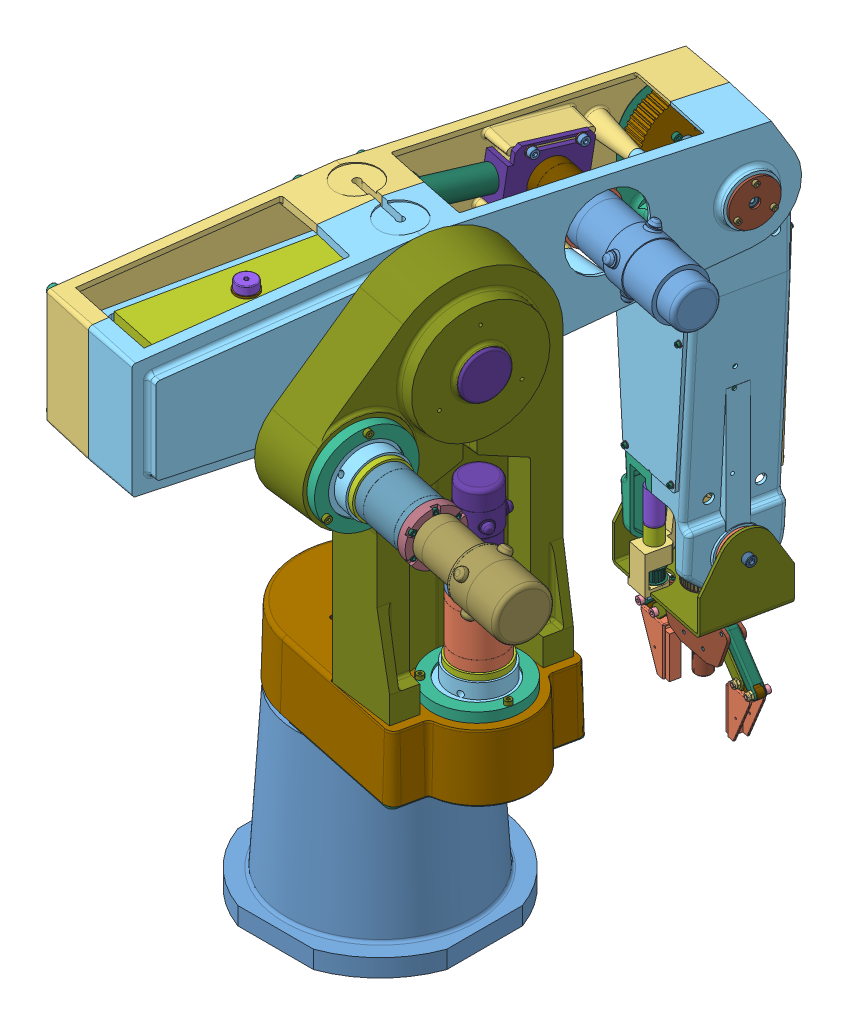
SolidWorks assembly Robot 2, configuration Défaut. Lengths in mm.
Overall size (465.28 616.21 608.92).
349 component instances, 132 part files, 24 mates.
Components (placement in the parent):
- Ens_Socle-1: Ens_Socle [Défaut] at origin size (212.48 231.5 219.24)
  - Socle-1: Socle [Default] at origin size (212.48 180 219.24)
  - Fourreau_200-604-1: Fourreau_200-604 [Défaut] at (0 176.5 0) x (-0.083866 0 0.996477) z (-0.996477 0 -0.083866) size (96 55 96)
  - CHC-M6_20-1: CHC-M6_20 [ISO 4762 M6 x 20 --- 20C] at (3.6062 156 -42.8485) x (0 1 0) z (-0.546944 0 0.837169) size (26 10 10)
  - poulie lacet-1: poulie lacet [Défaut] at (0 206.5 0) x (0.433454 0 0.901176) z (0 1 0) size (124 124 27)
  - Rondelle M6-1: Rondelle M6 [Washer ISO 7089 - 6] at (-35.9297 209 -24.5216) x (0 -1 0) z (0 0 1) size (1.6 12 12)
  - CHC-M6_25-1: CHC-M6_25 [ISO 4762 M6 x 25 --- 25C] at (-35.9297 216.6 -24.5216) x (0 -1 0) z (0.040163 0 0.999193) size (31 10 10)
  - Couvercle_300-732-1: Couvercle_300-732 [Défaut] at (0 175.5 0) x (-0.570868 0 0.821042) z (-0.821042 0 -0.570868) size (65 10.5 65)
  - CHC-M4_16-1: CHC-M4_16 [ISO 4762 M4 x 16 --- 16C] at (25.3374 166.5 -11.917) x (0 1 0) z (-0.937005 0 0.349316) size (20 7 7)
  - CHC-M4_16-2: CHC-M4_16 [ISO 4762 M4 x 16 --- 16C] at (-22.9892 166.5 -15.9843) x (0 1 0) z (0.771019 0 0.636812) size (20 7 7)
  - CHC-M4_16-3: CHC-M4_16 [ISO 4762 M4 x 16 --- 16C] at (-2.3482 166.5 27.9014) x (0 1 0) z (0.165986 0 -0.986128) size (20 7 7)
  - CHC-M6_25-2: CHC-M6_25 [ISO 4762 M6 x 25 --- 25C] at (-3.2715 216.6 43.3768) x (0 -1 0) z (0.845245 0 -0.534379) size (31 10 10)
  - CHC-M6_25-3: CHC-M6_25 [ISO 4762 M6 x 25 --- 25C] at (39.2011 216.6 -18.8552) x (0 -1 0) z (-0.885408 0 -0.464814) size (31 10 10)
  - Rondelle M6-2: Rondelle M6 [Washer ISO 7089 - 6] at (-3.2715 209 43.3768) x (0 -1 0) z (0.866025 0 -0.5) size (1.6 12 12)
  - Rondelle M6-3: Rondelle M6 [Washer ISO 7089 - 6] at (39.2011 209 -18.8552) x (0 -1 0) z (-0.866025 0 -0.5) size (1.6 12 12)
  - CHC-M6_20-2: CHC-M6_20 [ISO 4762 M6 x 20 --- 20C] at (-38.911 156 18.3012) x (0 1 0) z (0.998482 0 0.055083) size (26 10 10)
  - CHC-M6_20-3: CHC-M6_20 [ISO 4762 M6 x 20 --- 20C] at (35.3048 156 24.5473) x (0 1 0) z (-0.451538 0 -0.892252) size (26 10 10)
- SE_Chaise-1: SE_Chaise [Défaut] at (0 253.5 0) x (0.204064 0 -0.978958) z (0 -1 0) size (256.43 420.65 448.71)
  - SE-Assise-1: SE-Assise [Défaut] at origin size (171.51 268.51 86)
    - Assise_100-032-1: Assise_100-032 [Default] at origin size (171.51 268.51 67)
    - Axe_200-464-1: Axe_200-464 [Défaut] at (0 0 11.5) x (0 0 1) z (1 0 0) size (76 96 96)
    - Goupille Çlastique , 6x20-1: Goupille Çlastique , 6x20 [Défaut] at (-40 0 10) x (1 0 0) z (0 -1 0) size (5.98 20 6)
    - Goupille Çlastique , 6x20-2: Goupille Çlastique , 6x20 [Défaut] at (40 0 10) x (1 0 0) z (0 -1 0) size (5.98 20 6)
    - visFHC M6-16-1: visFHC M6-16 [B18.3.5M - 6 x 1.0 x 16 Socket FCHS  -- 16S] at (0 -42 0) x (0 0 1) z (-1 0 0) size (16 11.7 11.7)
    - visFHC M6-16-2: visFHC M6-16 [B18.3.5M - 6 x 1.0 x 16 Socket FCHS  -- 16S] at (-36.3731 21 0) x (0 0 1) z (0.5 0.866025 0) size (16 11.7 11.7)
    - visFHC M6-16-3: visFHC M6-16 [B18.3.5M - 6 x 1.0 x 16 Socket FCHS  -- 16S] at (36.3731 21 0) x (0 0 1) z (0.5 -0.866025 0) size (16 11.7 11.7)
    - SKF_7204-1: SKF_7204 [SKF - 7204 BE - 10,DE,NC,10_68] at (0 0 31) x (0 0 1) z (-1 0 0) size (14 47 47)
    - SKF_7204-2: SKF_7204 [SKF - 7204 BE - 10,DE,NC,10_68] at (0 0 67.5) x (0 0 -1) z (1 0 0) size (14 47 47)
    - Entrtoise_200-006-1: Entrtoise_200-006 [Default] at (0 0 38) x (1 0 0) z (0 -1 0) size (47 22.5 47)
    - Capot_201-294-1: Capot_201-294 [Défaut] at (0 0.5 67) size (170 180.5 2)
  - Dossier-1: Dossier [Défaut] at (-0.0064 64.9972 -279) x (1 0 0) z (0 1 0) size (234.27 388.58 71.5)
  - Moto-rÇducteur lacet-1: Moto-rÇducteur lacet [Défaut] at (2.5917 125.4972 -183.1) x (0 0 -1) z (0.5 0.866025 0) size (236.28 90 90)
    - Corps moto-rÇducteur-1: Corps moto-rÇducteur [Default] at origin size (199.6 50 51)
      - Moteur Parvex RS120G-1: Moteur Parvex RS120G [Défaut] at origin size (126 39.96 39.96)
      - Vis CHC M4x10-1: Vis CHC M4x10 [Défaut] at (-91.1 0 22) x (0 0 1) z (-1 0 0) size (7 7 14)
      - Entretoise-m-r-1: Entretoise-m-r [Défaut] at (-92.6 0 0) size (59.8 50 50)
      - RÇducteur Harmonic Drive HDUC 14 1U-CC-1: RÇducteur Harmonic Drive HDUC 14 1U-CC [Défaut] at (-92.6 0 0) size (123.2 50 50)
      - Vis CHC M4x10-2: Vis CHC M4x10 [Défaut] at (-91.1 -19.0526 11) x (0 -0.866025 0.5) z (-1 0 0) size (7 7 14)
      - Vis CHC M4x10-3: Vis CHC M4x10 [Défaut] at (-91.1 -19.0526 -11) x (0 -0.866025 -0.5) z (-1 0 0) size (7 7 14)
      - Vis CHC M4x10-4: Vis CHC M4x10 [Défaut] at (-91.1 0 -22) x (0 0 -1) z (-1 0 0) size (7 7 14)
      - Vis CHC M4x10-5: Vis CHC M4x10 [Défaut] at (-91.1 19.0526 -11) x (0 0.866025 -0.5) z (-1 0 0) size (7 7 14)
      - Vis CHC M4x10-6: Vis CHC M4x10 [Défaut] at (-91.1 19.0526 11) x (0 0.866025 0.5) z (-1 0 0) size (7 7 14)
      - Vis CHC M4-6-1: Vis CHC M4-6 [Défaut] at (-90.1 9.8995 9.8995) x (0 0 -1) z (1 0 0) size (6 6 10)
      - Vis CHC M4-6-2: Vis CHC M4-6 [Défaut] at (-90.1 -9.8995 9.8995) x (0 1 0) z (1 0 0) size (6 6 10)
      - Vis CHC M4-6-3: Vis CHC M4-6 [Défaut] at (-90.1 -9.8995 -9.8995) x (0 0 1) z (1 0 0) size (6 6 10)
      - Vis CHC M4-6-4: Vis CHC M4-6 [Défaut] at (-90.1 9.8995 -9.8995) x (0 -1 0) z (1 0 0) size (6 6 10)
      - Arbre de sortie-1: Arbre de sortie [Défaut] at (-159.6 0 0) size (40 8 8)
    - Palier-1: Palier [Défaut] at (-162.6 0 0) size (88.18 90 90)
      - Porte poulie motrice-1: Porte poulie motrice [Défaut] at origin size (73.68 74 74)
      - Bride-1: Bride [Défaut] at (-22.5 3 0) x (0 0 -1) z (-1 0 0) size (90 90 10)
      - Flasque-1: Flasque [Défaut] at (6 0 0) x (0 -0.664186 0.747567) z (-1 0 0) size (54 54 6)
      - VisCHC M4-40-1: VisCHC M4-40 [Défaut] at (-36 -16.2635 16.2635) x (0 0.997296 -0.073485) z (1 0 0) size (7 7 44)
      - VisCHC M4-40-2: VisCHC M4-40 [Défaut] at (-36 16.2635 16.2635) x (0 -0.073485 -0.997296) z (1 0 0) size (7 7 44)
      - VisCHC M4-40-3: VisCHC M4-40 [Défaut] at (-36 16.2635 -16.2635) x (0 -0.997296 0.073485) z (1 0 0) size (7 7 44)
      - VisCHC M4-40-4: VisCHC M4-40 [Défaut] at (-36 -16.2635 -16.2635) x (0 0.073485 0.997296) z (1 0 0) size (7 7 44)
      - anneau Çlastique int d32-1: anneau Çlastique int d32 [Défaut] at (-48.6 0 0) x (0 0 1) z (-1 0 0) size (33.7 32.99 1.2)
      - Vis CHC M4x10-1: Vis CHC M4x10 [Défaut] at (4.5 20 0) x (0 0 -1) z (1 0 0) size (7 7 14)
      - Vis CHC M4x10-2: Vis CHC M4x10 [Défaut] at (4.5 10 17.3205) x (0 0.866025 -0.5) z (1 0 0) size (7 7 14)
      - Vis CHC M4x10-3: Vis CHC M4x10 [Défaut] at (4.5 -10 17.3205) x (0 0.866025 0.5) z (1 0 0) size (7 7 14)
      - Vis CHC M4x10-4: Vis CHC M4x10 [Défaut] at (4.5 -20 0) x (0 0 1) z (1 0 0) size (7 7 14)
      - Vis CHC M4x10-5: Vis CHC M4x10 [Défaut] at (4.5 -10 -17.3205) x (0 -0.866025 0.5) z (1 0 0) size (7 7 14)
      - Vis CHC M4x10-6: Vis CHC M4x10 [Défaut] at (4.5 10 -17.3205) x (0 -0.866025 -0.5) z (1 0 0) size (7 7 14)
    - SKF 6002-1: SKF 6002 [SKF - 6002 - 12,DE,NC,12_68] at (-206.7 0 0) size (9 32 32)
    - SKF 6002-2: SKF 6002 [SKF - 6002 - 12,DE,NC,12_68] at (-185.6 0 0) size (9 32 32)
  - vis CHC M6-25-1: vis CHC M6-25 [ISO 4762 M6 x 25 --- 25S] at (-57.0064 122.9972 16) x (0 0 -1) z (-0.036606 -0.99933 0) size (31 10 10)
  - vis CHC M6-25-2: vis CHC M6-25 [ISO 4762 M6 x 25 --- 25S] at (-57.0064 77.9972 16) x (0 0 -1) z (-0.036606 -0.99933 0) size (31 10 10)
  - vis CHC M6-25-3: vis CHC M6-25 [ISO 4762 M6 x 25 --- 25S] at (56.9936 122.9972 16) x (0 0 -1) z (-0.036606 -0.99933 0) size (31 10 10)
  - vis CHC M6-25-4: vis CHC M6-25 [ISO 4762 M6 x 25 --- 25S] at (56.9936 77.9972 16) x (0 0 -1) z (-0.036606 -0.99933 0) size (31 10 10)
  - Goupille Çlastique , 6x20-1: Goupille Çlastique , 6x20 [Défaut] at (66.9936 122.9972 2) x (1 0 0) z (0 -1 0) size (5.98 20 6)
  - Goupille Çlastique , 6x20-2: Goupille Çlastique , 6x20 [Défaut] at (-42.0064 77.9972 2) x (1 0 0) z (0 -1 0) size (5.98 20 6)
  - Moteur Epaule-1: Moteur Epaule [Défaut] at (-95.2692 334.8972 -221) x (0 1 0) z (0.162984 0 0.986629) size (264.08 126.67 126.67)
    - Moteur RS210-1: Moteur RS210 [Défaut] at origin size (135.4 52 52)
    - entretoise-m-r bras-1: entretoise-m-r bras [Défaut] at (-120.4 0 0) x (1 0 0) z (0 0.162984 0.986629) size (59.8 54 54)
    - RÇducteur Harmonic Drive bras-1: RÇducteur Harmonic Drive bras [Défaut] at (-120.4 0 0) x (1 0 0) z (0 0.634463 0.772953) size (123.2 51.79 50)
    - Vis CHC M4x10-1: Vis CHC M4x10 [Défaut] at (-117.9 11.3806 8.1537) x (0 0.924309 0.381646) z (1 0 0) size (7 7 14)
    - Vis CHC M4x10-2: Vis CHC M4x10 [Défaut] at (-117.9 -8.1537 11.3806) x (0 -0.381646 0.924309) z (1 0 0) size (7 7 14)
    - Vis CHC M4x10-3: Vis CHC M4x10 [Défaut] at (-117.9 -11.3806 -8.1537) x (0 -0.924309 -0.381646) z (1 0 0) size (7 7 14)
    - Vis CHC M4x10-4: Vis CHC M4x10 [Défaut] at (-117.9 8.1537 -11.3806) x (0 0.381646 -0.924309) z (1 0 0) size (7 7 14)
    - Vis CHC M3-10-1: Vis CHC M3-10 [Défaut] at (-118.9 3.5857 21.7058) x (0 -0.692088 -0.721813) z (-1 0 0) size (5.5 5.5 13)
    - Vis CHC M3-10-2: Vis CHC M3-10 [Défaut] at (-118.9 -17.005 13.9582) x (0 0.279064 -0.960272) z (-1 0 0) size (5.5 5.5 13)
    - Vis CHC M3-10-3: Vis CHC M3-10 [Défaut] at (-118.9 -20.5906 -7.7476) x (0 0.971152 -0.238459) z (-1 0 0) size (5.5 5.5 13)
    - Vis CHC M3-10-4: Vis CHC M3-10 [Défaut] at (-118.9 -3.5857 -21.7058) x (0 0.692088 0.721813) z (-1 0 0) size (5.5 5.5 13)
    - Vis CHC M3-10-5: Vis CHC M3-10 [Défaut] at (-118.9 17.005 -13.9582) x (0 -0.279064 0.960272) z (-1 0 0) size (5.5 5.5 13)
    - Vis CHC M3-10-6: Vis CHC M3-10 [Défaut] at (-118.9 20.5906 7.7476) x (0 -0.971152 0.238459) z (-1 0 0) size (5.5 5.5 13)
    - Palier-1: Palier [Défaut] at (-190.4 0 0) x (1 0 0) z (0 0.634463 0.772953) size (88.18 90 90)
      - Porte poulie motrice-1: Porte poulie motrice [Défaut] at origin size (73.68 74 74)
      - Bride-1: Bride [Défaut] at (-22.5 3 0) x (0 0 -1) z (-1 0 0) size (90 90 10)
      - Flasque-1: Flasque [Défaut] at (6 0 0) x (0 -0.664186 0.747567) z (-1 0 0) size (54 54 6)
      - VisCHC M4-40-1: VisCHC M4-40 [Défaut] at (-36 -16.2635 16.2635) x (0 0.997296 -0.073485) z (1 0 0) size (7 7 44)
      - VisCHC M4-40-2: VisCHC M4-40 [Défaut] at (-36 16.2635 16.2635) x (0 -0.073485 -0.997296) z (1 0 0) size (7 7 44)
      - VisCHC M4-40-3: VisCHC M4-40 [Défaut] at (-36 16.2635 -16.2635) x (0 -0.997296 0.073485) z (1 0 0) size (7 7 44)
      - VisCHC M4-40-4: VisCHC M4-40 [Défaut] at (-36 -16.2635 -16.2635) x (0 0.073485 0.997296) z (1 0 0) size (7 7 44)
      - anneau Çlastique int d32-1: anneau Çlastique int d32 [Défaut] at (-48.6 0 0) x (0 0 1) z (-1 0 0) size (33.7 32.99 1.2)
      - Vis CHC M4x10-1: Vis CHC M4x10 [Défaut] at (4.5 20 0) x (0 0 -1) z (1 0 0) size (7 7 14)
      - Vis CHC M4x10-2: Vis CHC M4x10 [Défaut] at (4.5 10 17.3205) x (0 0.866025 -0.5) z (1 0 0) size (7 7 14)
      - Vis CHC M4x10-3: Vis CHC M4x10 [Défaut] at (4.5 -10 17.3205) x (0 0.866025 0.5) z (1 0 0) size (7 7 14)
      - Vis CHC M4x10-4: Vis CHC M4x10 [Défaut] at (4.5 -20 0) x (0 0 1) z (1 0 0) size (7 7 14)
      - Vis CHC M4x10-5: Vis CHC M4x10 [Défaut] at (4.5 -10 -17.3205) x (0 -0.866025 0.5) z (1 0 0) size (7 7 14)
      - Vis CHC M4x10-6: Vis CHC M4x10 [Défaut] at (4.5 10 -17.3205) x (0 -0.866025 -0.5) z (1 0 0) size (7 7 14)
    - SKF 6002-1: SKF 6002 [SKF - 6002 - 12,DE,NC,12_68] at (-213.4 0 0) size (9 32 32)
    - SKF 6002-2: SKF 6002 [SKF - 6002 - 12,DE,NC,12_68] at (-234.5 0 0) size (9 32 32)
  - Vis_CHC_M4-16-1: Vis_CHC_M4-16 [ISO 4762 M4 x 12 --- 12C] at (-133.3743 135.9972 -202) x (0 -1 0) z (0 0 1) size (20 7 7)
  - Vis_CHC_M4-16-2: Vis_CHC_M4-16 [ISO 4762 M4 x 12 --- 12C] at (-0.0064 167.9972 -12) x (0 0 1) z (0 1 0) size (20 7 7)
  - Vis_CHC_M4-16-3: Vis_CHC_M4-16 [ISO 4762 M4 x 12 --- 12C] at (-35.5134 106.4972 -12) x (0 0 1) z (-0.866025 -0.5 0) size (20 7 7)
  - Vis_CHC_M4-16-4: Vis_CHC_M4-16 [ISO 4762 M4 x 12 --- 12C] at (35.5007 106.4972 -12) x (0 0 1) z (0.866025 -0.5 0) size (20 7 7)
  - Vis_CHC_M4-16-5: Vis_CHC_M4-16 [ISO 4762 M4 x 12 --- 12C] at (-97.8672 135.9972 -263.5) x (0 -1 0) z (-0.866025 0 -0.5) size (20 7 7)
  - Vis_CHC_M4-16-6: Vis_CHC_M4-16 [ISO 4762 M4 x 12 --- 12C] at (-62.3602 135.9972 -202) x (0 -1 0) z (0.866025 0 -0.5) size (20 7 7)
  - Bouchon-1: Bouchon [Défaut] at (-0.0064 133.9972 -279) size (46 5.5 46)
  - Couvercle_301-396-1: Couvercle_301-396 [Défaut] at (-0.0064 71.9972 -279) x (0.866025 0 0.5) z (-0.5 0 0.866025) size (66 8 66)
  - Vis_CHC_M4-16-7: Vis_CHC_M4-16 [ISO 4762 M4 x 12 --- 12C] at (-0.0064 71.9972 -307.5) x (0 1 0) z (-0.976883 0 -0.213777) size (20 7 7)
  - Vis_CHC_M4-16-8: Vis_CHC_M4-16 [ISO 4762 M4 x 12 --- 12C] at (-24.6881 71.9972 -264.75) x (0 1 0) z (0.303305 0 0.952894) size (20 7 7)
  - Vis_CHC_M4-16-9: Vis_CHC_M4-16 [ISO 4762 M4 x 12 --- 12C] at (24.6754 71.9972 -264.75) x (0 1 0) z (0.673578 0 -0.739117) size (20 7 7)
  - Ecrou Ö encoches, M 17-1: Ecrou Ö encoches, M 17 [Défaut] at (0 0 75.5) x (-0.99693 -0.078302 0) z (-0.078302 0.99693 0) size (27.71 5 27.71)
  - Rondelle frein de 17-1: Rondelle frein de 17 [Défaut] at (0 0 74.5) x (-0.99693 -0.078302 0) z (-0.078302 0.99693 0) size (33.42 5.39 32.18)
- Bras-1: Bras [Défaut] at (-3.3238 505.7717 6.1308) x (-0.204064 0 0.978958) z (-0.978958 0 -0.204064) size (576.57 148.84 242.4)
  - BrasDroit-2: BrasDroit [Défaut] at origin size (576.57 148.84 66)
  - GoupillePosition-1: GoupillePosition [Défaut] at (-30.6737 92.2283 0) x (0 0 1) z (-1 0 0) size (10 8 8)
  - GoupillePosition-3: GoupillePosition [Défaut] at (234.3263 -27.2717 0) x (0 0 1) z (-1 0 0) size (10 8 8)
  - GoupillePosition-4: GoupillePosition [Défaut] at (-227.6737 51.7283 0) x (0 0 1) z (-1 0 0) size (10 8 8)
  - BrasGauche-2: BrasGauche [Défaut] at (-6.6737 26.7283 0) size (576.57 148.84 101.36)
  - Vis C HC, M 6x70-1: Vis C HC, M 6x70 [Défaut] at (-227.6737 51.7283 55) x (-0.629032 0.777379 0) z (0.777379 0.629032 0) size (10 76 10)
  - Vis C HC, M 6x70-7: Vis C HC, M 6x70 [Défaut] at (-30.6737 92.2283 55) x (0.427468 -0.90403 0) z (-0.90403 -0.427468 0) size (10 76 10)
  - Vis C HC, M 6x70-9: Vis C HC, M 6x70 [Défaut] at (234.3263 -27.2717 55) x (0.427468 -0.90403 0) z (-0.90403 -0.427468 0) size (10 76 10)
  - Vis C HC, M 6x70-11: Vis C HC, M 6x70 [Défaut] at (-165.6737 -17.2717 55) x (0.427468 -0.90403 0) z (-0.90403 -0.427468 0) size (10 76 10)
  - Vis C HC, M 6x70-15: Vis C HC, M 6x70 [Défaut] at (234.3263 77.7283 55) x (0.427468 -0.90403 0) z (-0.90403 -0.427468 0) size (10 76 10)
  - Vis C HC, M 6x70-21: Vis C HC, M 6x70 [Défaut] at (23.3263 91.126 55) x (0.427468 -0.90403 0) z (-0.90403 -0.427468 0) size (10 76 10)
  - Vis C HC, M 6x70-23: Vis C HC, M 6x70 [Défaut] at (-6.6737 -38.7717 55) x (0.427468 -0.90403 0) z (-0.90403 -0.427468 0) size (10 76 10)
  - contre_poids-1: contre_poids [Défaut] at (123.9539 42.7283 -46) size (175 60 60)
  - Vis C HC, M 8x70-1: Vis C HC, M 8x70 [Défaut] at (117.4539 78.7283 -16) x (0.870431 0 -0.492291) z (0.492291 0 0.870431) size (20 78.34 20)
  - Rondelle L, 8-1: Rondelle L, 8 [Défaut] at (117.4539 75.7283 -16) size (22 1.5 22)
  - Rondelle L, 8-3: Rondelle L, 8 [Défaut] at (117.4539 77.2283 -16) size (22 1.5 22)
  - SKF_6001-1: SKF_6001 [SKF - 6001 - 10,DE,NC,10_68] at (-286.6737 26.7283 -58) x (0 0 -1) z (1 0 0) size (8 28 28)
  - Couvercle_M300-013-1: Couvercle_M300-013 [Défaut] at (-286.6737 26.7283 -64) x (0 0 1) z (-1 0 0) size (4.5 45 45)
  - CHC_M3-10-1: CHC_M3-10 [ISO 4762 M3 x 10 --- 10C] at (-302.2622 17.7283 -69.5) x (0 0 1) z (-1 0 0) size (13 5.5 5.5)
  - CHC_M3-10-3: CHC_M3-10 [ISO 4762 M3 x 10 --- 10C] at (-286.6737 44.7283 -69.5) x (0 0 1) z (-1 0 0) size (13 5.5 5.5)
  - CHC_M3-10-9: CHC_M3-10 [ISO 4762 M3 x 10 --- 10C] at (-271.0852 17.7283 -69.5) x (0 0 1) z (-1 0 0) size (13 5.5 5.5)
  - Verin-pince-1: Verin-pince [Défaut] at (-48.6737 7.2342 -0.5445) x (-1 0 0) z (0 -0.130938 0.991391) size (269.69 47.71 50)
    - Support-verin-1: Support-verin [Défaut] at origin size (170 44 50)
    - 5079 DSN-25-80-1: 5079 DSN-25-80 [Défaut] at (-118.1875 36.1693 13.898) x (0 -0.972057 -0.234746) z (1 0 0) size (36.95 32 205.57)
      - Corps-1: Corps [Défaut] at (13.1476 11.1224 0) size (27 27 173.5)
      - Piston-1: Piston [Défaut] at (13.1476 11.1224 4.0685) size (25 25 177.5)
      - Ecrou-1: Ecrou [Défaut] at (13.1476 11.1224 2.0036) size (36.95 32 11)
  - CHC_M3-10-10: CHC_M3-10 [ISO 4762 M3 x 10 --- 10C] at (106.3263 -1.975 9.6121) x (0 0.991391 0.130938) z (0 -0.130938 0.991391) size (13 5.5 5.5)
  - CHC_M3-10-11: CHC_M3-10 [ISO 4762 M3 x 10 --- 10C] at (106.3263 0.8402 -11.7028) x (0 0.991391 0.130938) z (-0.130938 -0.129811 0.982855) size (13 5.5 5.5)
  - SupportMoteur_M300-005-1: SupportMoteur_M300-005 [Défaut] at (-166.3149 43.5192 23.5) x (-0.988512 -0.151141 0) z (0 0 -1) size (75 70 28)
  - Rondelle Z, 3-1: Rondelle Z, 3 [Défaut] at (106.3263 0.9992 10.0049) x (1 0 0) z (0 -0.130938 0.991391) size (6 0.8 6)
  - Rondelle Z, 3-3: Rondelle Z, 3 [Défaut] at (106.3263 3.8144 -11.31) x (1 0 0) z (0 -0.130938 0.991391) size (6 0.8 6)
  - VisCHC_M5-16-1: VisCHC_M5-16 [ISO 4762 M5 x 16 --- 16C] at (-149.3329 75.8068 12.5) x (0 0 1) z (-0.747365 -0.664413 0) size (21 8.5 8.5)
  - VisCHC_M5-16-3: VisCHC_M5-16 [ISO 4762 M5 x 16 --- 16C] at (-141.3413 15.8945 12.5) x (0 0 1) z (-1 0 0) size (21 8.5 8.5)
  - VisCHC_M5-16-5: VisCHC_M5-16 [ISO 4762 M5 x 16 --- 16C] at (-185.0651 10.9723 12.5) x (0 0 1) z (-1 0 0) size (21 8.5 8.5)
  - VisCHC_M5-16-7: VisCHC_M5-16 [ISO 4762 M5 x 16 --- 16C] at (-193.005 70.4446 12.5) x (0 0 1) z (-1 0 0) size (21 8.5 8.5)
  - Rondelle Z, 5-1: Rondelle Z, 5 [Défaut] at (-185.0651 10.9723 18.5) x (1 0 0) z (0 1 0) size (10 1 10)
  - Rondelle Z, 5-3: Rondelle Z, 5 [Défaut] at (-193.005 70.4446 18.5) x (1 0 0) z (0 1 0) size (10 1 10)
  - Rondelle Z, 5-5: Rondelle Z, 5 [Défaut] at (-149.3329 75.8068 18.5) x (1 0 0) z (0 1 0) size (10 1 10)
  - Rondelle Z, 5-7: Rondelle Z, 5 [Défaut] at (-141.3413 15.8945 18.5) x (1 0 0) z (0 1 0) size (10 1 10)
  - AXE_Bras-1: AXE_Bras [Défaut] at (-6.6737 26.7283 -80) x (0 0 -1) z (-1 0 0) size (72.5 126.04 126.04)
    - AXE_M300-010-1: AXE_M300-010 [Défaut] at origin size (72.5 98 98)
    - Poulie_M300-014-1: Poulie_M300-014 [Défaut] at (-4 0 0) size (30 126.04 126.04)
    - Vic_CHCM6-16-1: Vic_CHCM6-16 [ISO 4762 M6 x 16 --- 16C] at (9.2 22 -38.1051) x (-1 0 0) z (0 0.831566 -0.555426) size (22 10 10)
    - Goupille6-32-1: Goupille6-32 [Parallel Pin ISO 8734 - 6 x 32 - A - St] at (-14 44 0) size (32 6 6)
    - Goupille6-32-2: Goupille6-32 [Parallel Pin ISO 8734 - 6 x 32 - A - St] at (-14 -31.1127 31.1127) x (1 0 0) z (0 -0.90193 0.431882) size (32 6 6)
    - EntretoiseM200-006-1: EntretoiseM200-006 [Défaut] at (35.5 0 0) x (1 0 0) z (0 -0.984877 -0.173252) size (21.5 47 47)
    - 7204_Rlt-Billes-1: 7204_Rlt-Billes [SKF - 7204 BE - 10,DE,NC,10_68] at (7 0 0) x (1 0 0) z (0 -0.825996 0.563676) size (14 47 47)
    - 7204_Rlt-Billes-2: 7204_Rlt-Billes [SKF - 7204 BE - 10,DE,NC,10_68] at (42.5 0 0) x (-1 0 0) z (0 -0.662732 0.748856) size (14 47 47)
    - Ecrou Ö encoches, M 20-1: Ecrou Ö encoches, M 20 [Défaut] at (50.5 0 0) x (0 0.493503 -0.869744) z (0 -0.869744 -0.493503) size (31.75 7.06 31.75)
    - Rondelle frein de 20-1: Rondelle frein de 20 [Défaut] at (49.5 0 0) x (0 0.317084 0.948397) z (0 0.948397 -0.317084) size (36.64 6.14 35.22)
    - Rondelle M, 6-1: Rondelle M, 6 [Défaut] at (2 22 -38.1051) x (0 -0.99765 -0.068521) z (0 -0.068521 0.99765) size (14 1.2 14)
    - Vic_CHCM6-16-2: Vic_CHCM6-16 [ISO 4762 M6 x 16 --- 16C] at (9.2 -44 0) x (-1 0 0) z (0 -0.896796 -0.442445) size (22 10 10)
    - Vic_CHCM6-16-3: Vic_CHCM6-16 [ISO 4762 M6 x 16 --- 16C] at (9.2 22 38.1051) x (-1 0 0) z (0 0.06523 0.99787) size (22 10 10)
    - Rondelle M, 6-2: Rondelle M, 6 [Défaut] at (2 -44 0) x (0 0.439484 0.89825) z (0 0.89825 -0.439484) size (14 1.2 14)
    - Rondelle M, 6-3: Rondelle M, 6 [Défaut] at (2 22 38.1051) x (0 0.558165 -0.82973) z (0 -0.82973 -0.558165) size (14 1.2 14)
  - Rondelle M, 6-1: Rondelle M, 6 [Défaut] at (-6.6737 -3.0038 -59) x (1 0 0) z (0 -1 0) size (14 1.2 14)
  - Rondelle M, 6-3: Rondelle M, 6 [Défaut] at (-32.4225 41.5944 -59) x (1 0 0) z (0 -1 0) size (14 1.2 14)
  - Rondelle M, 6-5: Rondelle M, 6 [Défaut] at (19.0751 41.5944 -59) x (1 0 0) z (0 -1 0) size (14 1.2 14)
  - Vic_CHCM6-16-7: Vic_CHCM6-16 [ISO 4762 M6 x 16 --- 16C] at (-32.4225 41.5944 -51.8) x (0 0 -1) z (1 0 0) size (22 10 10)
  - Vic_CHCM6-16-9: Vic_CHCM6-16 [ISO 4762 M6 x 16 --- 16C] at (-6.6737 -3.0038 -51.8) x (0 0 -1) z (1 0 0) size (22 10 10)
  - Vic_CHCM6-16-11: Vic_CHCM6-16 [ISO 4762 M6 x 16 --- 16C] at (19.0751 41.5944 -51.8) x (0 0 -1) z (-1 0 0) size (22 10 10)
  - parallel pin unhardened_iso-1: parallel pin unhardened_iso [Parallel Pin ISO 2338 - 6 m6 x 20 - St] at (-6.6737 56.7283 -73) x (0 0 1) z (0.997282 0.073675 0) size (20 6 6)
  - parallel pin unhardened_iso-3: parallel pin unhardened_iso [Parallel Pin ISO 2338 - 6 m6 x 20 - St] at (14.5395 5.5151 -73) x (0 0 1) z (0.997282 0.073675 0) size (20 6 6)
  - Couvercle_M300-013-4: Couvercle_M300-013 [Défaut] at (-286.6737 26.7283 63) x (0 0 -1) z (1 0 0) size (4.5 45 45)
  - Rondelle Çpaisse Z, 12-1: Rondelle Çpaisse Z, 12 [Défaut] at (-286.6737 26.7283 -50.5) x (0.066998 0.997753 0) z (-0.997753 0.066998 0) size (15 3.5 15)
  - SKF_6001-2: SKF_6001 [SKF - 6001 - 10,DE,NC,10_68] at (-286.6737 26.7283 57) x (0 0 -1) z (0.798379 0.602155 0) size (8 28 28)
  - Rondelle Çpaisse Z, 12-3: Rondelle Çpaisse Z, 12 [Défaut] at (-286.6737 26.7283 49.5) x (0.444076 -0.895989 0) z (-0.895989 -0.444076 0) size (15 3.5 15)
  - CHC_M3-10-14: CHC_M3-10 [ISO 4762 M3 x 10 --- 10C] at (-271.0852 17.7283 68.5) x (0 0 -1) z (1 0 0) size (13 5.5 5.5)
  - CHC_M3-10-16: CHC_M3-10 [ISO 4762 M3 x 10 --- 10C] at (-302.2622 17.7283 68.5) x (0 0 -1) z (1 0 0) size (13 5.5 5.5)
  - CHC_M3-10-18: CHC_M3-10 [ISO 4762 M3 x 10 --- 10C] at (-286.6737 44.7283 68.5) x (0 0 -1) z (1 0 0) size (13 5.5 5.5)
  - AXE 04 021 M300 011-1: AXE 04 021 M300 011 [Défaut] at (-286.6737 26.7283 -63) x (-0.545711 0.837974 0) z (0 0 1) size (12 12 125)
  - Vis Ö bille M6-40-1: Vis Ö bille M6-40 [Défaut] at (-37.2131 63.2586 37.5) x (-0.988512 -0.151141 0) z (0.079359 -0.519031 0.851063) size (106.14 36 36)
    - socket head cap screw_iso-1: socket head cap screw_iso [PreviewCfg] at origin size (104 36 36)
    - Bille-1: Bille [Défaut] at (103.5 0 0) x (-0.326721 -0.900194 0.28793) z (-0.943911 0.295385 -0.147577) size (4 4 4)
  - hex nut gradec_iso-1: hex nut gradec_iso [Hexagon Nut ISO - 4034 - M6 - N] at (-120.7445 50.4869 37.5) x (0.022844 -0.149405 -0.988512) z (0.988512 0.151141 0) size (10 11.55 6.1)
  - MotoReduc_Coude-1: MotoReduc_Coude [Défaut] at (-166.3149 43.5192 -32.5) x (0 0 -1) z (0.805857 -0.592111 0) size (233.4 63.14 63.14)
    - RÇducteur Harmonic Drive HDUC 11 1U-CC-1: RÇducteur Harmonic Drive HDUC 11 1U-CC [Défaut] at origin size (123.2 40 40)
    - Moteur Parvex RS220F-1: Moteur Parvex RS220F [Défaut] at (141.4 0 0) x (1 0 0) z (0 0.244629 0.969617) size (210.51 52 52)
    - BrideCoude-1: BrideCoude [Défaut] at (-5 0 0) size (10 52 52)
    - Sortie reduc-1: Sortie reduc [Défaut] at (-52 0 0) size (40 10 10)
  - socket head cap screw_iso-1: socket head cap screw_iso [ISO 4762 M4 x 8 --- 8N] at (-149.016 46.1642 27) x (0 0 -1) z (0.779732 0.626114 0) size (12 7 7)
  - Rondelle, W 4-1: Rondelle, W 4 [Défaut] at (-149.016 46.1642 23) x (0 -1 0) z (1 0 0) size (7.3 1.5 7.3)
  - Rondelle, W 4-2: Rondelle, W 4 [Défaut] at (-168.9599 60.8182 23) x (1 0 0) z (0 1 0) size (7.3 1.5 7.3)
  - Rondelle, W 4-3: Rondelle, W 4 [Défaut] at (-183.6139 40.8743 23) x (0 1 0) z (-1 0 0) size (7.3 1.5 7.3)
  - Rondelle, W 4-4: Rondelle, W 4 [Défaut] at (-163.67 26.2203 23) x (-1 0 0) z (0 -1 0) size (7.3 1.5 7.3)
  - socket head cap screw_iso-2: socket head cap screw_iso [ISO 4762 M4 x 8 --- 8N] at (-168.9599 60.8182 27) x (0 0 -1) z (-0.626114 0.779732 0) size (12 7 7)
  - socket head cap screw_iso-3: socket head cap screw_iso [ISO 4762 M4 x 8 --- 8N] at (-183.6139 40.8743 27) x (0 0 -1) z (-0.779732 -0.626114 0) size (12 7 7)
  - socket head cap screw_iso-4: socket head cap screw_iso [ISO 4762 M4 x 8 --- 8N] at (-163.67 26.2203 27) x (0 0 -1) z (0.626114 -0.779732 0) size (12 7 7)
